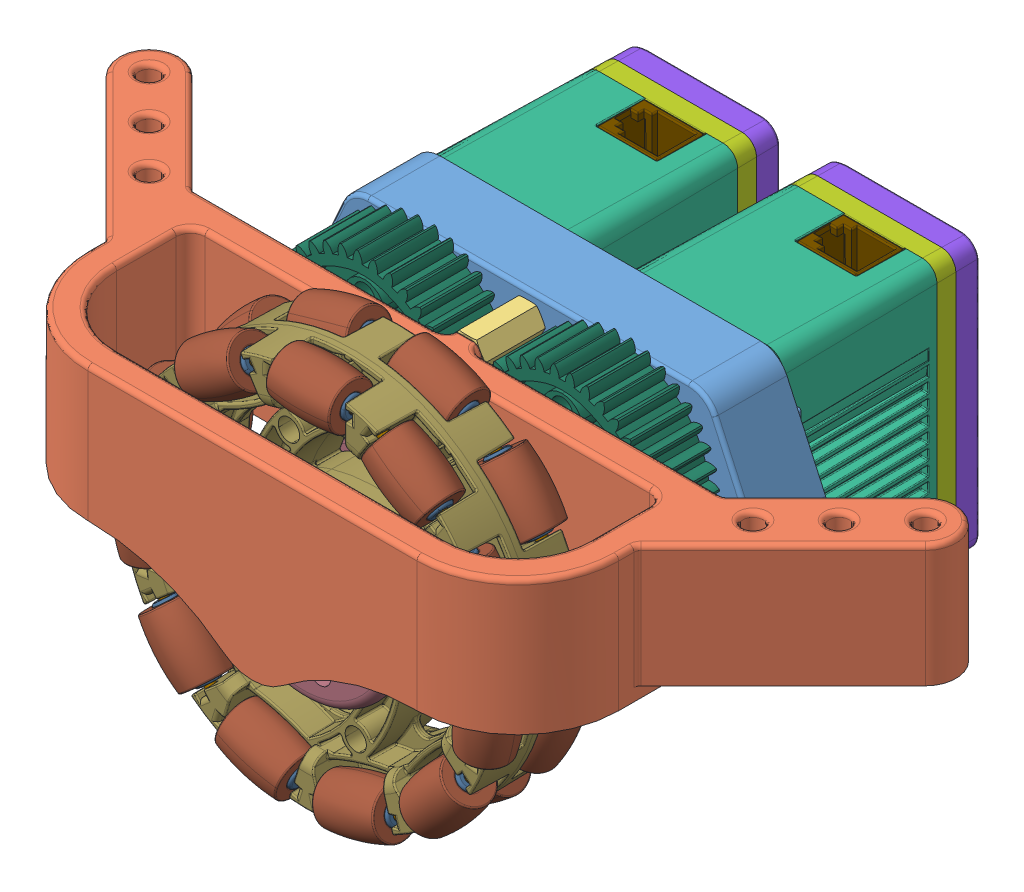
SolidWorks assembly Holo_Module_Assembly, configuration Default. Lengths in mm.
Overall size (174.34 110.57 117.06).
164 component instances, 28 part files, 47 mates.
Components (placement in the parent):
- Holo_Module-1: Holo_Module [Default] at (11.0032 60.106 76.6942) size (94.5 52.1 17)
- Gearbox_and_Wheel_Hub-1: Gearbox_and_Wheel_Hub [Default] at (31.7532 47.106 113.4442) x (-1 0 0) z (0 0 -1) size (174.34 39.65 65.67)
- 1_2_ Standoff (275-1014)-1: 1_2_ Standoff (275-1014) [Default] at (31.7532 72.106 83.0442) x (1 0 0) z (0 1 0) size (7.34 12.7 7.34)
- 1_2_ Standoff (275-1014)-2: 1_2_ Standoff (275-1014) [Default] at (-11.4968 51.106 83.0442) x (1 0 0) z (0 1 0) size (7.34 12.7 7.34)
- 1_2_ Standoff (275-1014)-3: 1_2_ Standoff (275-1014) [Default] at (75.0032 51.106 83.0442) x (1 0 0) z (0 1 0) size (7.34 12.7 7.34)
- 0.25in 0.375in OD Nylon Spacer-1: 0.25in 0.375in OD Nylon Spacer [Default] at (31.7532 45.4568 91.3942) x (1 0 0) z (0 -1 0) size (9.53 6.35 9.53)
- 0.25in 0.375in OD Nylon Spacer-2: 0.25in 0.375in OD Nylon Spacer [Default] at (31.7532 45.4568 76.6942) x (0.551769 -0.833997 0) z (0.833997 0.551769 0) size (9.53 6.35 9.53)
- 0.125in 0.375in OD Nylon Spacer-1: 0.125in 0.375in OD Nylon Spacer [Default] at (11.0032 60.106 94.5692) x (1 0 0) z (0 1 0) size (9.53 3.17 9.53)
- 0.125in 0.375in OD Nylon Spacer-2: 0.125in 0.375in OD Nylon Spacer [Default] at (52.5032 60.106 94.5692) x (1 0 0) z (0 1 0) size (9.53 3.17 9.53)
- 0.125in 0.375in OD Nylon Spacer-3: 0.125in 0.375in OD Nylon Spacer [Default] at (31.7532 45.4568 131.3192) x (-0.923728 -0.383049 0) z (0.383049 -0.923728 0) size (9.53 3.17 9.53)
- Drive Shaft 60mm-1: Drive Shaft 60mm [Default] at (31.7532 45.4568 -21.0808) x (0.707001 0.707212 0) z (0 0 1) size (3.28 3.28 60)
- #8-32 x 1_2_ Star Drive Screw (276-4992)-2: #8-32 x 1_2_ Star Drive Screw (276-4992) [Default] at (31.7532 72.106 97.7442) x (-0.923728 -0.383049 0) z (-0.383049 0.923728 0) size (7.92 14.91 7.92)
- #8-32 x 1_2_ Star Drive Screw (276-4992)-3: #8-32 x 1_2_ Star Drive Screw (276-4992) [Default] at (75.0032 51.106 97.7442) x (-0.923728 -0.383049 0) z (-0.383049 0.923728 0) size (7.92 14.91 7.92)
- #8-32 x 1_2_ Star Drive Screw (276-4992)-4: #8-32 x 1_2_ Star Drive Screw (276-4992) [Default] at (-11.4968 51.106 97.7442) x (-0.923728 -0.383049 0) z (-0.383049 0.923728 0) size (7.92 14.91 7.92)
- #8-32 x 7_8_ Star Drive Screw (276-4995)-2: #8-32 x 7_8_ Star Drive Screw (276-4995) [Default] at (-11.4968 51.106 61.6942) x (1 0 0) z (0 1 0) size (7.92 24.44 7.92)
- #8-32 x 7_8_ Star Drive Screw (276-4995)-3: #8-32 x 7_8_ Star Drive Screw (276-4995) [Default] at (31.7532 72.106 61.6942) x (1 0 0) z (0 1 0) size (7.92 24.44 7.92)
- #8-32 x 7_8_ Star Drive Screw (276-4995)-4: #8-32 x 7_8_ Star Drive Screw (276-4995) [Default] at (75.0032 51.106 61.6942) x (1 0 0) z (0 1 0) size (7.92 24.44 7.92)
- Holo_Module_Omni_Wheel_Assembly-1: Holo_Module_Omni_Wheel_Assembly [Default] at (37.7219 100.2583 39.0679) x (-0.961777 -0.273835 0) z (0 0 1) size (90.82 89.11 34)
  - 3.25_ Omni-Directional Wheel (276-3526) part-1: 3.25_ Omni-Directional Wheel (276-3526) part [Default] at (20.7471 51.0724 74.1563) size (90.82 89.11 34)
    - 3.25_ Omni-Directional Wheel (276-3526) .step-1: 3.25_ Omni-Directional Wheel (276-3526) .step [Default] at origin size (90.82 89.11 34)
      - Roller Assembly.step-1: Roller Assembly.step [Default] at (-0.0014 35.9575 7.1) x (0 0.963098 -0.269151) z (-1 0 0) size (14.05 14.05 18.75)
        - 276-3526-001 Rev 1.step-1: 276-3526-001 Rev 1.step [Default] at origin size (2 2 18.75)
        - 276-3526-003 Rev 1.step-1: 276-3526-003 Rev 1.step [Default] at origin size (6.15 6.15 14.2)
        - 276-3526-002 Rev 1.step-1: 276-3526-002 Rev 1.step [Default] x (0 0 1) z (-0.908956 0.416893 0) size (13.2 10.6 10.6)
      - Roller Assembly.step-2: Roller Assembly.step [Default] at (-19.4287 30.2567 7.1) x (0.421057 -0.655178 0.627258) z (-0.841254 -0.540641 0) size (14.05 14.05 18.75)
        - 276-3526-001 Rev 1.step-1: 276-3526-001 Rev 1.step [Default] at origin size (2 2 18.75)
        - 276-3526-003 Rev 1.step-1: 276-3526-003 Rev 1.step [Default] at origin size (6.15 6.15 14.2)
        - 276-3526-002 Rev 1.step-1: 276-3526-002 Rev 1.step [Default] x (0 0 1) z (-0.908956 0.416893 0) size (13.2 10.6 10.6)
      - Roller Assembly.step-3: Roller Assembly.step [Default] at (-35.5935 -5.1038 7.1) x (0.979746 0.140866 -0.142315) z (0.142315 -0.989821 0) size (14.05 14.05 18.75)
        - 276-3526-001 Rev 1.step-1: 276-3526-001 Rev 1.step [Default] at origin size (2 2 18.75)
        - 276-3526-003 Rev 1.step-1: 276-3526-003 Rev 1.step [Default] at origin size (6.15 6.15 14.2)
        - 276-3526-002 Rev 1.step-1: 276-3526-002 Rev 1.step [Default] x (0 0 1) z (-0.908956 0.416893 0) size (13.2 10.6 10.6)
      - Roller Assembly.step-4: Roller Assembly.step [Default] at (-10.1434 -34.4972 7.1) x (0.079373 0.27032 -0.959493) z (0.959493 -0.281733 0) size (14.05 14.05 18.75)
        - 276-3526-001 Rev 1.step-1: 276-3526-001 Rev 1.step [Default] at origin size (2 2 18.75)
        - 276-3526-003 Rev 1.step-1: 276-3526-003 Rev 1.step [Default] at origin size (6.15 6.15 14.2)
        - 276-3526-002 Rev 1.step-1: 276-3526-002 Rev 1.step [Default] x (0 0 1) z (-0.908956 0.416893 0) size (13.2 10.6 10.6)
      - Roller Assembly.step-5: Roller Assembly.step [Default] at (27.166 -23.5574 7.1) x (-0.355209 0.30779 -0.882662) z (0.654861 0.75575 0) size (14.05 14.05 18.75)
        - 276-3526-001 Rev 1.step-1: 276-3526-001 Rev 1.step [Default] at origin size (2 2 18.75)
        - 276-3526-003 Rev 1.step-1: 276-3526-003 Rev 1.step [Default] at origin size (6.15 6.15 14.2)
        - 276-3526-002 Rev 1.step-1: 276-3526-002 Rev 1.step [Default] x (0 0 1) z (-0.908956 0.416893 0) size (13.2 10.6 10.6)
      - Roller Assembly.step-6: Roller Assembly.step [Default] at (32.7138 14.9249 7.1) x (0.89908 0.410596 0.151875) z (-0.415415 0.909632 0) size (14.05 14.05 18.75)
        - 276-3526-001 Rev 1.step-1: 276-3526-001 Rev 1.step [Default] at origin size (2 2 18.75)
        - 276-3526-003 Rev 1.step-1: 276-3526-003 Rev 1.step [Default] at origin size (6.15 6.15 14.2)
        - 276-3526-002 Rev 1.step-1: 276-3526-002 Rev 1.step [Default] x (0 0 1) z (-0.908956 0.416893 0) size (13.2 10.6 10.6)
      - Roller Assembly.step-7: Roller Assembly.step [Default] at (19.4515 30.242 7.1) x (0.194707 0.302971 0.932898) z (-0.841254 0.540641 0) size (14.05 14.05 18.75)
        - 276-3526-001 Rev 1.step-1: 276-3526-001 Rev 1.step [Default] at origin size (2 2 18.75)
        - 276-3526-003 Rev 1.step-1: 276-3526-003 Rev 1.step [Default] at origin size (6.15 6.15 14.2)
        - 276-3526-002 Rev 1.step-1: 276-3526-002 Rev 1.step [Default] x (0 0 1) z (-0.908956 0.416893 0) size (13.2 10.6 10.6)
      - Roller Assembly.step-8: Roller Assembly.step [Default] at (-32.7025 14.9497 7.1) x (0.82743 -0.377875 0.415415) z (-0.415415 -0.909632 0) size (14.05 14.05 18.75)
        - 276-3526-001 Rev 1.step-1: 276-3526-001 Rev 1.step [Default] at origin size (2 2 18.75)
        - 276-3526-003 Rev 1.step-1: 276-3526-003 Rev 1.step [Default] at origin size (6.15 6.15 14.2)
        - 276-3526-002 Rev 1.step-1: 276-3526-002 Rev 1.step [Default] x (0 0 1) z (-0.908956 0.416893 0) size (13.2 10.6 10.6)
      - Roller Assembly.step-9: Roller Assembly.step [Default] at (-27.1838 -23.5369 7.1) x (0.578931 0.501646 -0.642799) z (0.654861 -0.75575 0) size (14.05 14.05 18.75)
        - 276-3526-001 Rev 1.step-1: 276-3526-001 Rev 1.step [Default] at origin size (2 2 18.75)
        - 276-3526-003 Rev 1.step-1: 276-3526-003 Rev 1.step [Default] at origin size (6.15 6.15 14.2)
        - 276-3526-002 Rev 1.step-1: 276-3526-002 Rev 1.step [Default] x (0 0 1) z (-0.908956 0.416893 0) size (13.2 10.6 10.6)
      - Roller Assembly.step-10: Roller Assembly.step [Default] at (10.1174 -34.5048 7.1) x (0.079373 -0.27032 -0.959493) z (0.959493 0.281733 0) size (14.05 14.05 18.75)
        - 276-3526-001 Rev 1.step-1: 276-3526-001 Rev 1.step [Default] at origin size (2 2 18.75)
        - 276-3526-003 Rev 1.step-1: 276-3526-003 Rev 1.step [Default] at origin size (6.15 6.15 14.2)
        - 276-3526-002 Rev 1.step-1: 276-3526-002 Rev 1.step [Default] x (0 0 1) z (-0.908956 0.416893 0) size (13.2 10.6 10.6)
      - Roller Assembly.step-11: Roller Assembly.step [Default] at (35.5896 -5.1307 7.1) x (0.988515 -0.142127 -0.05136) z (0.142315 0.989821 0) size (14.05 14.05 18.75)
        - 276-3526-001 Rev 1.step-1: 276-3526-001 Rev 1.step [Default] at origin size (2 2 18.75)
        - 276-3526-003 Rev 1.step-1: 276-3526-003 Rev 1.step [Default] at origin size (6.15 6.15 14.2)
        - 276-3526-002 Rev 1.step-1: 276-3526-002 Rev 1.step [Default] x (0 0 1) z (-0.908956 0.416893 0) size (13.2 10.6 10.6)
      - Roller Assembly.step-12: Roller Assembly.step [Default] at (10.1434 34.4972 -7.1) x (0.083119 0.283078 -0.955489) z (0.959493 -0.281733 0) size (14.05 14.05 18.75)
        - 276-3526-001 Rev 1.step-1: 276-3526-001 Rev 1.step [Default] at origin size (2 2 18.75)
        - 276-3526-003 Rev 1.step-1: 276-3526-003 Rev 1.step [Default] at origin size (6.15 6.15 14.2)
        - 276-3526-002 Rev 1.step-1: 276-3526-002 Rev 1.step [Default] x (0 0 1) z (-0.908956 0.416893 0) size (13.2 10.6 10.6)
      - Roller Assembly.step-13: Roller Assembly.step [Default] at (27.1838 23.5369 -7.1) x (0.582526 0.504762 -0.637086) z (0.654861 -0.75575 0) size (14.05 14.05 18.75)
        - 276-3526-001 Rev 1.step-1: 276-3526-001 Rev 1.step [Default] at origin size (2 2 18.75)
        - 276-3526-003 Rev 1.step-1: 276-3526-003 Rev 1.step [Default] at origin size (6.15 6.15 14.2)
        - 276-3526-002 Rev 1.step-1: 276-3526-002 Rev 1.step [Default] x (0 0 1) z (-0.908956 0.416893 0) size (13.2 10.6 10.6)
      - Roller Assembly.step-14: Roller Assembly.step [Default] at (35.5935 5.1038 -7.1) x (0.926341 0.133188 -0.352355) z (0.142315 -0.989821 0) size (14.05 14.05 18.75)
        - 276-3526-001 Rev 1.step-1: 276-3526-001 Rev 1.step [Default] at origin size (2 2 18.75)
        - 276-3526-003 Rev 1.step-1: 276-3526-003 Rev 1.step [Default] at origin size (6.15 6.15 14.2)
        - 276-3526-002 Rev 1.step-1: 276-3526-002 Rev 1.step [Default] x (0 0 1) z (-0.908956 0.416893 0) size (13.2 10.6 10.6)
      - Roller Assembly.step-15: Roller Assembly.step [Default] at (32.7025 -14.9497 -7.1) x (0.897398 -0.409828 0.163453) z (-0.415415 -0.909632 0) size (14.05 14.05 18.75)
        - 276-3526-001 Rev 1.step-1: 276-3526-001 Rev 1.step [Default] at origin size (2 2 18.75)
        - 276-3526-003 Rev 1.step-1: 276-3526-003 Rev 1.step [Default] at origin size (6.15 6.15 14.2)
        - 276-3526-002 Rev 1.step-1: 276-3526-002 Rev 1.step [Default] x (0 0 1) z (-0.908956 0.416893 0) size (13.2 10.6 10.6)
      - Roller Assembly.step-16: Roller Assembly.step [Default] at (19.4287 -30.2567 -7.1) x (0.277612 -0.431972 0.858098) z (-0.841254 -0.540641 0) size (14.05 14.05 18.75)
        - 276-3526-001 Rev 1.step-1: 276-3526-001 Rev 1.step [Default] at origin size (2 2 18.75)
        - 276-3526-003 Rev 1.step-1: 276-3526-003 Rev 1.step [Default] at origin size (6.15 6.15 14.2)
        - 276-3526-002 Rev 1.step-1: 276-3526-002 Rev 1.step [Default] x (0 0 1) z (-0.908956 0.416893 0) size (13.2 10.6 10.6)
      - Roller Assembly.step-17: Roller Assembly.step [Default] at (-0.0136 -35.9575 -7.1) x (0 -0.239919 0.970793) z (-1 0 0) size (14.05 14.05 18.75)
        - 276-3526-001 Rev 1.step-1: 276-3526-001 Rev 1.step [Default] at origin size (2 2 18.75)
        - 276-3526-003 Rev 1.step-1: 276-3526-003 Rev 1.step [Default] at origin size (6.15 6.15 14.2)
        - 276-3526-002 Rev 1.step-1: 276-3526-002 Rev 1.step [Default] x (0 0 1) z (-0.908956 0.416893 0) size (13.2 10.6 10.6)
      - Roller Assembly.step-18: Roller Assembly.step [Default] at (-19.4515 -30.242 -7.1) x (0.31008 0.482494 0.819176) z (-0.841254 0.540641 0) size (14.05 14.05 18.75)
        - 276-3526-001 Rev 1.step-1: 276-3526-001 Rev 1.step [Default] at origin size (2 2 18.75)
        - 276-3526-003 Rev 1.step-1: 276-3526-003 Rev 1.step [Default] at origin size (6.15 6.15 14.2)
        - 276-3526-002 Rev 1.step-1: 276-3526-002 Rev 1.step [Default] x (0 0 1) z (-0.908956 0.416893 0) size (13.2 10.6 10.6)
      - Roller Assembly.step-19: Roller Assembly.step [Default] at (-32.7138 -14.9249 -7.1) x (0.58758 0.268339 0.763377) z (-0.415415 0.909632 0) size (14.05 14.05 18.75)
        - 276-3526-001 Rev 1.step-1: 276-3526-001 Rev 1.step [Default] at origin size (2 2 18.75)
        - 276-3526-003 Rev 1.step-1: 276-3526-003 Rev 1.step [Default] at origin size (6.15 6.15 14.2)
        - 276-3526-002 Rev 1.step-1: 276-3526-002 Rev 1.step [Default] x (0 0 1) z (-0.908956 0.416893 0) size (13.2 10.6 10.6)
      - Roller Assembly.step-20: Roller Assembly.step [Default] at (-35.5896 5.1307 -7.1) x (0.965498 -0.138818 0.220323) z (0.142315 0.989821 0) size (14.05 14.05 18.75)
        - 276-3526-001 Rev 1.step-1: 276-3526-001 Rev 1.step [Default] at origin size (2 2 18.75)
        - 276-3526-003 Rev 1.step-1: 276-3526-003 Rev 1.step [Default] at origin size (6.15 6.15 14.2)
        - 276-3526-002 Rev 1.step-1: 276-3526-002 Rev 1.step [Default] x (0 0 1) z (-0.908956 0.416893 0) size (13.2 10.6 10.6)
      - Roller Assembly.step-21: Roller Assembly.step [Default] at (-27.166 23.5574 -7.1) x (0.75327 -0.652712 -0.080935) z (0.654861 0.75575 0) size (14.05 14.05 18.75)
        - 276-3526-001 Rev 1.step-1: 276-3526-001 Rev 1.step [Default] at origin size (2 2 18.75)
        - 276-3526-003 Rev 1.step-1: 276-3526-003 Rev 1.step [Default] at origin size (6.15 6.15 14.2)
        - 276-3526-002 Rev 1.step-1: 276-3526-002 Rev 1.step [Default] x (0 0 1) z (-0.908956 0.416893 0) size (13.2 10.6 10.6)
      - Roller Assembly.step-22: Roller Assembly.step [Default] at (-10.1174 34.5048 -7.1) x (0.123782 -0.421563 -0.898311) z (0.959493 0.281733 0) size (14.05 14.05 18.75)
        - 276-3526-001 Rev 1.step-1: 276-3526-001 Rev 1.step [Default] at origin size (2 2 18.75)
        - 276-3526-003 Rev 1.step-1: 276-3526-003 Rev 1.step [Default] at origin size (6.15 6.15 14.2)
        - 276-3526-002 Rev 1.step-1: 276-3526-002 Rev 1.step [Default] x (0 0 1) z (-0.908956 0.416893 0) size (13.2 10.6 10.6)
      - 276-3526-004 Rev 1.step-1: 276-3526-004 Rev 1.step [Default] at origin size (78.5 78.5 19.07)
  - Wheel_Spacer-1: Wheel_Spacer [Default] at (20.7471 51.0724 80.5063) size (38.1 38.1 7.3)
  - Wheel_Spacer-2: Wheel_Spacer [Default] at (20.7471 51.0724 67.8063) x (1 0 0) z (0 0 -1) size (38.1 38.1 7.3)
  - Metal Shaft Inserts (276-3881-002)-1: Metal Shaft Inserts (276-3881-002) [Default] at (20.7471 51.0724 89.0763) x (1 0 0) z (0 1 0) size (10.03 5.08 10.03)
  - Metal Shaft Inserts (276-3881-002)-2: Metal Shaft Inserts (276-3881-002) [Default] at (20.7471 51.0724 59.2363) x (1 0 0) z (0 -1 0) size (10.03 5.08 10.03)
- 36T High Strength with Inserts-1: 36T High Strength with Inserts [Default] at (0.0709 26.4541 104.1462) x (0.999622 -0.027509 0) z (0.027509 0.999622 0) size (40.08 12.7 40.08)
  - 36T High Strength Gear (276-5034)-1: 36T High Strength Gear (276-5034) [Default] at (10.0025 20.102 33.9399) size (40.08 12.7 40.08)
  - Metal Shaft Inserts (276-3881-002)-1: Metal Shaft Inserts (276-3881-002) [Default] at (10.0279 13.952 33.9653) size (10.03 5.08 10.03)
  - Metal Shaft Inserts (276-3881-002)-2: Metal Shaft Inserts (276-3881-002) [Default] at (10.0279 26.252 33.9145) x (-1 0 0) z (0 0 1) size (10.03 5.08 10.03)
- 36T High Strength with Inserts-2: 36T High Strength with Inserts [Default] at (42.5007 26.1661 104.1462) x (1 0 0) z (0 1 0) size (40.08 12.7 40.08)
  - 36T High Strength Gear (276-5034)-1: 36T High Strength Gear (276-5034) [Default] at (10.0025 20.102 33.9399) size (40.08 12.7 40.08)
  - Metal Shaft Inserts (276-3881-002)-1: Metal Shaft Inserts (276-3881-002) [Default] at (10.0279 13.952 33.9653) size (10.03 5.08 10.03)
  - Metal Shaft Inserts (276-3881-002)-2: Metal Shaft Inserts (276-3881-002) [Default] at (10.0279 26.252 33.9145) x (-1 0 0) z (0 0 1) size (10.03 5.08 10.03)
- 12T High Strength Metal Pinion with HS hole (276-2251)-1: 12T High Strength Metal Pinion with HS hole (276-2251) [Default] at (31.7532 45.4568 84.0442) x (1 0 0) z (0 -1 0) size (14.8 12.7 14.8)
- V5 Smart Motor (276-4840) no cap-1: V5 Smart Motor (276-4840) no cap [Default] at (52.5032 47.406 44.4942) x (0 1 0) z (0 0 1) size (59.01 35.33 59.91)
  - V5 Smart Motor (276-4840).step-1: V5 Smart Motor (276-4840).step [Default] at origin size (59.01 35.33 59.91)
    - 276-4840-900 Rev6_Instruction.step-1: 276-4840-900 Rev6_Instruction.step [Default] at (-14.3 0 -17.2) size (52.79 15.94 38.15)
      - 276-4840-901 Rev6.step-1: 276-4840-901 Rev6.step [Default] at (10.75 -10.05 17.8) x (-1 0 0) z (0 0 1) size (49.9 1.6 38.15)
      - 276-4840-902 Rev2.step-1: 276-4840-902 Rev2.step [Default] at (31.25 -9.25 6.2) x (0 0 -1) z (0 -1 0) size (10.35 11.39 15.94)
      - 276-4840-022 Rev4.step-1: 276-4840-022 Rev4.step [Default] at (31.25 -9.25 6.2) x (0 0 -1) z (1 0 0) size (10.26 9.1 5.51)
    - 276-4840-110 Rev10_Instruction.step-1: 276-4840-110 Rev10_Instruction.step [Default] at (12.7 0 14.7) size (35.33 35.33 31.1)
      - 276-4840-061 Rev7_Ring_Gear_Fixed01 .6 Rev3.step-1: 276-4840-061 Rev7_Ring_Gear_Fixed01 .6 Rev3.step [Default] at origin size (28.79 28.39 24.6)
      - 276-4840-018 Rev6.step-1: 276-4840-018 Rev6.step [Default] at (0 0 6.7) x (-0.483174 0.875524 0) z (0 0 1) size (26 26 12.3)
      - 276-4840-059 Rev2.step-1: 276-4840-059 Rev2.step [Default] at (0 0 10.3) size (28.4 28.4 8.5)
      - 276-4840-062 Rev1.step-1: 276-4840-062 Rev1.step [Default] at (-12.1353 8.8168 12.3) x (0.956835 -0.290632 0) z (-0.290632 -0.956835 0) size (3.2 6.56 3.2)
      - 276-4840-062 Rev1.step-2: 276-4840-062 Rev1.step [Default] at (12.1353 8.8168 12.3) x (0.978427 0.206591 0) z (0.206591 -0.978427 0) size (3.2 6.56 3.2)
      - 276-4840-062 Rev1.step-3: 276-4840-062 Rev1.step [Default] at (-12.1353 -8.8168 12.3) x (0.72563 0.688086 0) z (0.688086 -0.72563 0) size (3.2 6.56 3.2)
    - 276-4840-001 Rev38.step-1: 276-4840-001 Rev38.step [Default] at origin size (57.3 33 46.9)
    - 276-4840-005 Rev27.step-1: 276-4840-005 Rev27.step [Default] at (0 0 -17.95) size (56.17 31.87 12.9)
    - 276-4840-004 Rev16.step-1: 276-4840-004 Rev16.step [Default] at (0 0 -19.2) size (56.01 31.71 9.21)
    - 276-4840-009 Rev3.step-1: 276-4840-009 Rev3.step [Default] at (25.45 13.5 15.7) x (0.19987 -0.979823 0) z (-0.979823 -0.19987 0) size (3.4 41.31 4.34)
    - 276-4840-009 Rev3.step-2: 276-4840-009 Rev3.step [Default] at (-25.45 -13.5 15.7) x (-0.998855 0.047836 0) z (0.047836 0.998855 0) size (3.4 41.31 4.34)
    - 276-4840-009 Rev3.step-3: 276-4840-009 Rev3.step [Default] at (25.45 -13.5 15.7) x (-0.975374 0.220559 0) z (0.220559 0.975374 0) size (3.4 41.31 4.34)
    - 276-4840-009 Rev3.step-4: 276-4840-009 Rev3.step [Default] at (-25.45 13.5 15.7) x (-0.922256 0.38658 0) z (0.38658 0.922256 0) size (3.4 41.31 4.34)
    - 276-4840-025 Rev19.step-1: 276-4840-025 Rev19.step [Default] at (12.7 0 -22.63) x (-0.993315 0.115437 0) z (0 0 1) size (14.82 14.83 35.18)
- V5 Smart Motor (276-4840) no cap-2: V5 Smart Motor (276-4840) no cap [Default] at (11.0032 47.406 44.4942) x (0 1 0) z (0 0 1) size (59.01 35.33 59.91)
  - V5 Smart Motor (276-4840).step-1: V5 Smart Motor (276-4840).step [Default] at origin size (59.01 35.33 59.91)
    - 276-4840-900 Rev6_Instruction.step-1: 276-4840-900 Rev6_Instruction.step [Default] at (-14.3 0 -17.2) size (52.79 15.94 38.15)
      - 276-4840-901 Rev6.step-1: 276-4840-901 Rev6.step [Default] at (10.75 -10.05 17.8) x (-1 0 0) z (0 0 1) size (49.9 1.6 38.15)
      - 276-4840-902 Rev2.step-1: 276-4840-902 Rev2.step [Default] at (31.25 -9.25 6.2) x (0 0 -1) z (0 -1 0) size (10.35 11.39 15.94)
      - 276-4840-022 Rev4.step-1: 276-4840-022 Rev4.step [Default] at (31.25 -9.25 6.2) x (0 0 -1) z (1 0 0) size (10.26 9.1 5.51)
    - 276-4840-110 Rev10_Instruction.step-1: 276-4840-110 Rev10_Instruction.step [Default] at (12.7 0 14.7) size (35.33 35.33 31.1)
      - 276-4840-061 Rev7_Ring_Gear_Fixed01 .6 Rev3.step-1: 276-4840-061 Rev7_Ring_Gear_Fixed01 .6 Rev3.step [Default] at origin size (28.79 28.39 24.6)
      - 276-4840-018 Rev6.step-1: 276-4840-018 Rev6.step [Default] at (0 0 6.7) x (-0.483174 0.875524 0) z (0 0 1) size (26 26 12.3)
      - 276-4840-059 Rev2.step-1: 276-4840-059 Rev2.step [Default] at (0 0 10.3) size (28.4 28.4 8.5)
      - 276-4840-062 Rev1.step-1: 276-4840-062 Rev1.step [Default] at (-12.1353 8.8168 12.3) x (0.956835 -0.290632 0) z (-0.290632 -0.956835 0) size (3.2 6.56 3.2)
      - 276-4840-062 Rev1.step-2: 276-4840-062 Rev1.step [Default] at (12.1353 8.8168 12.3) x (0.978427 0.206591 0) z (0.206591 -0.978427 0) size (3.2 6.56 3.2)
      - 276-4840-062 Rev1.step-3: 276-4840-062 Rev1.step [Default] at (-12.1353 -8.8168 12.3) x (0.72563 0.688086 0) z (0.688086 -0.72563 0) size (3.2 6.56 3.2)
    - 276-4840-001 Rev38.step-1: 276-4840-001 Rev38.step [Default] at origin size (57.3 33 46.9)
    - 276-4840-005 Rev27.step-1: 276-4840-005 Rev27.step [Default] at (0 0 -17.95) size (56.17 31.87 12.9)
    - 276-4840-004 Rev16.step-1: 276-4840-004 Rev16.step [Default] at (0 0 -19.2) size (56.01 31.71 9.21)
    - 276-4840-009 Rev3.step-1: 276-4840-009 Rev3.step [Default] at (25.45 13.5 15.7) x (0.19987 -0.979823 0) z (-0.979823 -0.19987 0) size (3.4 41.31 4.34)
    - 276-4840-009 Rev3.step-2: 276-4840-009 Rev3.step [Default] at (-25.45 -13.5 15.7) x (-0.998855 0.047836 0) z (0.047836 0.998855 0) size (3.4 41.31 4.34)
    - 276-4840-009 Rev3.step-3: 276-4840-009 Rev3.step [Default] at (25.45 -13.5 15.7) x (-0.975374 0.220559 0) z (0.220559 0.975374 0) size (3.4 41.31 4.34)
    - 276-4840-009 Rev3.step-4: 276-4840-009 Rev3.step [Default] at (-25.45 13.5 15.7) x (-0.922256 0.38658 0) z (0.38658 0.922256 0) size (3.4 41.31 4.34)
    - 276-4840-025 Rev19.step-1: 276-4840-025 Rev19.step [Default] at (12.7 0 -22.63) x (-0.993315 0.115437 0) z (0 0 1) size (14.82 14.83 35.18)
Mates (geometry in assembly coordinates):
- Concentric2: concentric aligned: cylinder of Holo_Module-1 through (-11.4968 51.106 61.6942) axis (0 0 1) radius 2.25; cylinder of Gearbox_and_Wheel_Hub-1 through (-11.4968 51.106 65.8459) axis (0 0 1) radius 2.25
- Concentric4: concentric aligned: cylinder of Holo_Module-1 through (75.0032 51.106 61.6942) axis (0 0 1) radius 2.25; cylinder of Gearbox_and_Wheel_Hub-1 through (75.0032 51.106 65.8459) axis (0 0 1) radius 2.25
- Concentric5: concentric anti-aligned: cylinder of Holo_Module-1 through (75.0032 51.106 61.6942) axis (0 0 1) radius 2.25; cylinder of 1_2_ Standoff (275-1014)-3 through (75.0032 51.106 89.3942) axis (0 0 -1) radius 2.0955
- Concentric6: concentric anti-aligned: cylinder of Holo_Module-1 through (31.7532 72.106 61.6942) axis (0 0 1) radius 2.25; cylinder of 1_2_ Standoff (275-1014)-1 through (31.7532 72.106 89.3942) axis (0 0 -1) radius 2.0955
- Concentric7: concentric anti-aligned: cylinder of Holo_Module-1 through (-11.4968 51.106 61.6942) axis (0 0 1) radius 2.25; cylinder of 1_2_ Standoff (275-1014)-2 through (-11.4968 51.106 89.3942) axis (0 0 -1) radius 2.0955
- Coincident1: coincident anti-aligned: plane of Holo_Module-1 through (11.0032 60.106 76.6942) normal (0 0 1); plane of 1_2_ Standoff (275-1014)-2 through (-13.3299 47.931 76.6942) normal (0 0 -1)
- Coincident2: coincident anti-aligned: plane of Holo_Module-1 through (11.0032 60.106 76.6942) normal (0 0 1); plane of 1_2_ Standoff (275-1014)-1 through (29.9201 68.931 76.6942) normal (0 0 -1)
- Coincident3: coincident anti-aligned: plane of Holo_Module-1 through (11.0032 60.106 76.6942) normal (0 0 1); plane of 1_2_ Standoff (275-1014)-3 through (73.1701 47.931 76.6942) normal (0 0 -1)
- Concentric12: concentric anti-aligned: circle of 0.125in 0.375in OD Nylon Spacer-3; circle of Gearbox_and_Wheel_Hub-1
- Coincident10: coincident anti-aligned: plane of Gearbox_and_Wheel_Hub-1 through (31.7532 45.4568 131.3192) normal (0 0 -1); plane of 0.125in 0.375in OD Nylon Spacer-3 through (31.7532 45.4568 131.3192) normal (0 0 1)
- Concentric13: concentric anti-aligned: circle of Gearbox_and_Wheel_Hub-1; circle of 0.125in 0.375in OD Nylon Spacer-1
- Coincident11: coincident anti-aligned: plane of Gearbox_and_Wheel_Hub-1 through (11.0032 60.106 94.5692) normal (0 0 -1); plane of 0.125in 0.375in OD Nylon Spacer-1 through (11.0032 60.106 94.5692) normal (0 0 1)
- Concentric14: concentric anti-aligned: circle of Gearbox_and_Wheel_Hub-1; circle of 0.125in 0.375in OD Nylon Spacer-2
- Coincident12: coincident anti-aligned: plane of Gearbox_and_Wheel_Hub-1 through (52.5032 60.106 94.5692) normal (0 0 -1); plane of 0.125in 0.375in OD Nylon Spacer-2 through (52.5032 60.106 94.5692) normal (0 0 1)
- Concentric15: concentric anti-aligned: cylinder of Gearbox_and_Wheel_Hub-1 through (31.7532 45.4568 65.8459) axis (0 0 1) radius 5; cylinder of 0.25in 0.375in OD Nylon Spacer-1 through (31.7532 45.4568 97.7442) axis (0 0 -1) radius 4.7625
- Coincident13: coincident aligned: plane of Gearbox_and_Wheel_Hub-1 through (31.7532 75.106 97.7442) normal (0 0 1); plane of 0.25in 0.375in OD Nylon Spacer-1 through (31.7532 45.4568 97.7442) normal (0 0 1)
- Concentric16: concentric anti-aligned: cylinder of Holo_Module-1 through (31.7532 45.4568 61.6942) axis (0 0 1) radius 5; circle of 0.25in 0.375in OD Nylon Spacer-2
- Coincident14: coincident anti-aligned: plane of Holo_Module-1 through (31.7532 45.4568 70.3442) normal (0 0 1); plane of 0.25in 0.375in OD Nylon Spacer-2 through (31.7532 45.4568 70.3442) normal (0 0 -1)
- Concentric17: concentric aligned: circle of 0.25in 0.375in OD Nylon Spacer-1; circle of Drive Shaft 60mm-1
- Coincident15: coincident anti-aligned: plane of Gearbox_and_Wheel_Hub-1 through (31.7532 45.4568 131.3192) normal (0 0 -1); plane of Drive Shaft 60mm-1 through (29.5082 45.4565 131.3192) normal (0 0 1)
- Concentric21: concentric aligned: cylinder of Gearbox_and_Wheel_Hub-1 through (31.7532 72.106 65.8459) axis (0 0 1) radius 2.25; cylinder of #8-32 x 1_2_ Star Drive Screw (276-4992)-2 through (31.7532 72.106 85.0442) axis (0 0 1) radius 2.0828
- Concentric22: concentric aligned: cylinder of Gearbox_and_Wheel_Hub-1 through (-11.4968 51.106 65.8459) axis (0 0 1) radius 2.25; cylinder of #8-32 x 1_2_ Star Drive Screw (276-4992)-4 through (-11.4968 51.106 85.0442) axis (0 0 1) radius 2.0828
- Concentric23: concentric aligned: cylinder of Gearbox_and_Wheel_Hub-1 through (75.0032 51.106 65.8459) axis (0 0 1) radius 2.25; cylinder of #8-32 x 1_2_ Star Drive Screw (276-4992)-3 through (75.0032 51.106 85.0442) axis (0 0 1) radius 2.0828
- Coincident19: coincident anti-aligned: plane of Gearbox_and_Wheel_Hub-1 through (31.7532 75.106 97.7442) normal (0 0 1); plane of #8-32 x 1_2_ Star Drive Screw (276-4992)-3 through (75.0032 51.106 97.7442) normal (0 0 -1)
- Coincident20: coincident anti-aligned: plane of Gearbox_and_Wheel_Hub-1 through (31.7532 75.106 97.7442) normal (0 0 1); plane of #8-32 x 1_2_ Star Drive Screw (276-4992)-2 through (31.7532 72.106 97.7442) normal (0 0 -1)
- Coincident21: coincident anti-aligned: plane of Gearbox_and_Wheel_Hub-1 through (31.7532 75.106 97.7442) normal (0 0 1); plane of #8-32 x 1_2_ Star Drive Screw (276-4992)-4 through (-11.4968 51.106 97.7442) normal (0 0 -1)
- Concentric24: concentric anti-aligned: cylinder of Holo_Module-1 through (-11.4968 51.106 61.6942) axis (0 0 1) radius 2.25; cylinder of #8-32 x 7_8_ Star Drive Screw (276-4995)-2 through (-11.4968 51.106 83.9192) axis (0 0 -1) radius 2.0828
- Concentric25: concentric anti-aligned: cylinder of Holo_Module-1 through (31.7532 72.106 61.6942) axis (0 0 1) radius 2.25; cylinder of #8-32 x 7_8_ Star Drive Screw (276-4995)-3 through (31.7532 72.106 83.9192) axis (0 0 -1) radius 2.0828
- Concentric26: concentric anti-aligned: cylinder of Holo_Module-1 through (75.0032 51.106 61.6942) axis (0 0 1) radius 2.25; cylinder of #8-32 x 7_8_ Star Drive Screw (276-4995)-4 through (75.0032 51.106 83.9192) axis (0 0 -1) radius 2.0828
- Coincident22: coincident anti-aligned: plane of Holo_Module-1 through (11.0032 60.106 61.6942) normal (0 0 -1); plane of #8-32 x 7_8_ Star Drive Screw (276-4995)-4 through (75.0032 51.106 61.6942) normal (0 0 1)
- Coincident23: coincident anti-aligned: plane of Holo_Module-1 through (11.0032 60.106 61.6942) normal (0 0 -1); plane of #8-32 x 7_8_ Star Drive Screw (276-4995)-3 through (31.7532 72.106 61.6942) normal (0 0 1)
- Coincident24: coincident anti-aligned: plane of Holo_Module-1 through (11.0032 60.106 61.6942) normal (0 0 -1); plane of #8-32 x 7_8_ Star Drive Screw (276-4995)-2 through (-11.4968 51.106 61.6942) normal (0 0 1)
- Concentric27: concentric aligned: circle of 0.125in 0.375in OD Nylon Spacer-3; circle of Holo_Module_Omni_Wheel_Assembly-1/Wheel_Spacer-1
- Concentric28: concentric aligned: cylinder of Holo_Module-1 through (52.5032 34.706 61.6942) axis (0 0 1) radius 4.1; circle of V5 Smart Motor (276-4840) no cap-1/V5 Smart Motor (276-4840).step-1/276-4840-001 Rev38.step-1
- Parallel1: parallel aligned: line of Holo_Module-1 through (61.0032 75.106 74.1942) axis (-1 0 0); line of V5 Smart Motor (276-4840) no cap-1/V5 Smart Motor (276-4840).step-1/276-4840-001 Rev38.step-1 through (65.4032 76.056 60.6942) axis (-1 0 0)
- Coincident27: coincident anti-aligned: plane of Holo_Module-1 through (11.0032 60.106 61.6942) normal (0 0 -1); plane of V5 Smart Motor (276-4840) no cap-1/V5 Smart Motor (276-4840).step-1/276-4840-001 Rev38.step-1 through (39.6032 22.356 61.6942) normal (0 0 1)
- Concentric29: concentric aligned: cylinder of Holo_Module-1 through (11.0032 34.706 61.6942) axis (0 0 1) radius 4.1; circle of V5 Smart Motor (276-4840) no cap-2/V5 Smart Motor (276-4840).step-1/276-4840-001 Rev38.step-1
- Parallel2: parallel anti-aligned: line of Holo_Module-1 through (19.5032 75.106 74.1942) axis (-1 0 0); line of V5 Smart Motor (276-4840) no cap-2/V5 Smart Motor (276-4840).step-1/276-4840-001 Rev38.step-1 through (-1.8968 18.756 60.6942) axis (1 0 0)
- Coincident29: coincident anti-aligned: plane of Holo_Module-1 through (11.0032 60.106 61.6942) normal (0 0 -1); plane of V5 Smart Motor (276-4840) no cap-2/V5 Smart Motor (276-4840).step-1/276-4840-001 Rev38.step-1 through (-1.8968 22.356 61.6942) normal (0 0 1)
- Concentric30: concentric anti-aligned: circle of 0.25in 0.375in OD Nylon Spacer-2; circle of 12T High Strength Metal Pinion with HS hole (276-2251)-1
- Distance1: distance = 1 mm anti-aligned: plane of 12T High Strength Metal Pinion with HS hole (276-2251)-1 through (32.5435 42.5093 90.3942) normal (0 0 1); plane of 0.25in 0.375in OD Nylon Spacer-1 through (31.7532 45.4568 91.3942) normal (0 0 -1)
- Concentric31: concentric anti-aligned: circle of Gearbox_and_Wheel_Hub-1; circle of 36T High Strength with Inserts-1/36T High Strength Gear (276-5034)-1
- Distance2: distance = 1 mm anti-aligned: plane of 36T High Strength with Inserts-1/36T High Strength Gear (276-5034)-1 through (1.9601 58.9783 90.3942) normal (0 0 1); plane of Gearbox_and_Wheel_Hub-1 through (31.7532 75.106 91.3942) normal (0 0 -1)
- Concentric32: concentric anti-aligned: circle of Gearbox_and_Wheel_Hub-1; circle of 36T High Strength with Inserts-2/36T High Strength Gear (276-5034)-1
- Distance3: distance = 1 mm anti-aligned: plane of 36T High Strength with Inserts-2/36T High Strength Gear (276-5034)-1 through (43.4945 58.73 90.3942) normal (0 0 1); plane of Gearbox_and_Wheel_Hub-1 through (31.7532 75.106 91.3942) normal (0 0 -1)
- Coincident30: coincident anti-aligned: plane of Gearbox_and_Wheel_Hub-1 through (31.7532 47.106 89.3942) normal (0 0 -1); plane of 1_2_ Standoff (275-1014)-2 through (-13.3299 47.931 89.3942) normal (0 0 1)
- Coincident31: coincident anti-aligned: plane of 0.125in 0.375in OD Nylon Spacer-3 through (31.7532 45.4568 128.1442) normal (0 0 -1); plane of Holo_Module_Omni_Wheel_Assembly-1/Metal Shaft Inserts (276-3881-002)-1 through (31.7532 45.4568 128.1442) normal (0 0 1)
